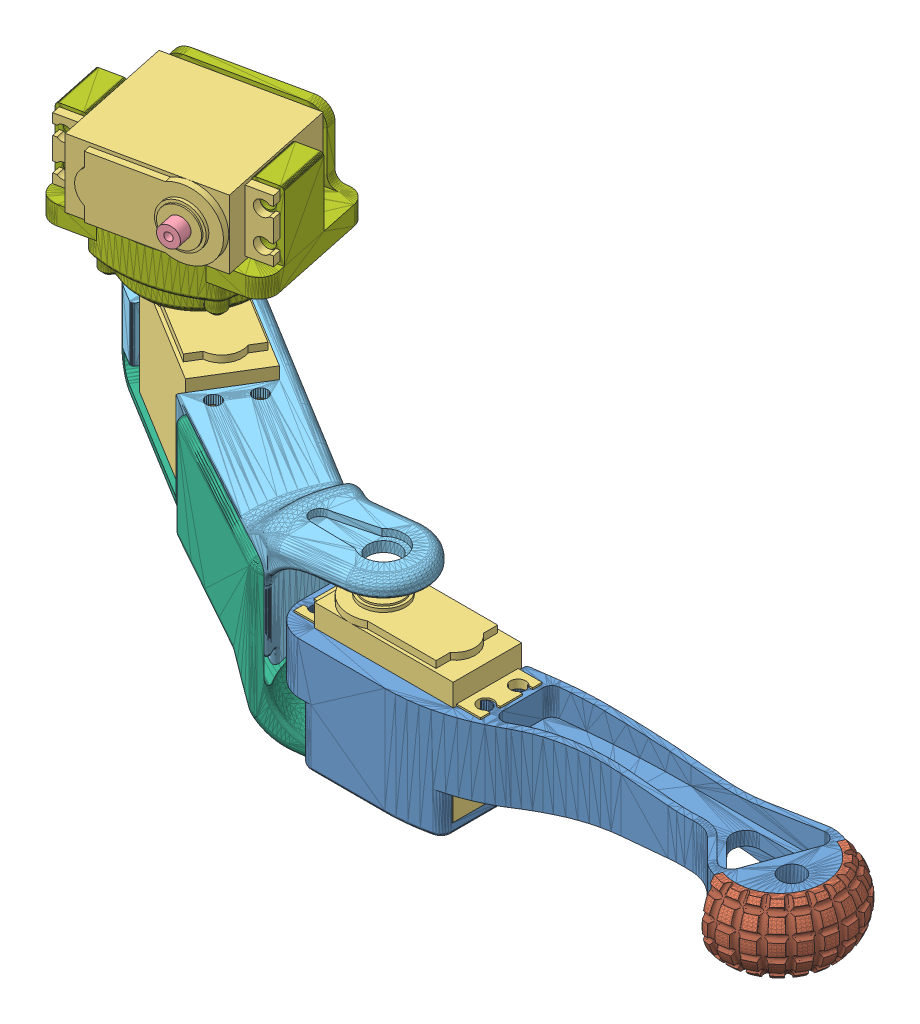
SolidWorks assembly left_foot_front, configuration Default. Lengths in mm.
Overall size (271.86 94.6 110.14).
14 component instances, 7 part files, 22 mates.
Components (placement in the parent):
- L_wrist_mg-1: L_wrist_mg [Default] at (-104.9134 49.2874 139.9903) size (149.99 36.9 30)
- foot-1: foot [Default] at (21.0866 19.2874 149.9903) x (0.342019 0 -0.939693) z (-0.939693 0 -0.342019) size (38.32 20 19.41)
- MG996R-1: MG996R [Default] at (-84.6634 -9.7126 149.9903) size (54.5 43 20)
  - servo-1: servo [Default] at origin size (54.5 39 20)
  - shaft-1: shaft [Default] at (-10.1089 43 0) x (-0.837169 0 -0.546944) z (-0.546944 0 0.837169) size (5.9 19.57 5.9)
- L_arm_mg-1: L_arm_mg [Default] at (-196.4399 30.2874 92.0951) x (-0.522898 0 0.852395) z (0.852395 0 0.522898) size (38.24 39.8 137.4)
- MG996R-2: MG996R [Default] at (-184.4079 -1.7126 111.2077) x (0.852395 0 0.522898) z (-0.522898 0 0.852395) size (54.5 43 20)
  - servo-1: servo [Default] at origin size (54.5 39 20)
  - shaft-1: shaft [Default] at (-10.1089 43 0) x (-0.837169 0 -0.546944) z (-0.546944 0 0.837169) size (5.9 19.57 5.9)
- L_arm_cover-1: L_arm_cover [Default] at (-199.5307 32.5874 83.7466) x (-0.522898 0 0.852395) z (0.852395 0 0.522898) size (41.16 45 143.55)
- MG996R-3: MG996R [Default] at (-196.3785 66.9874 90.0217) x (-0.978469 0 0.206392) z (0 1 0) size (54.5 43 20)
  - servo-1: servo [Default] at origin size (54.5 39 20)
  - shaft-1: shaft [Default] at (-10.1089 43 0) x (-0.837169 0 -0.546944) z (-0.546944 0 0.837169) size (5.9 19.57 5.9)
- R_arm_joint_mg-1: R_arm_joint_mg [Default] at (-214.9542 106.9874 100.0719) x (0 1 0) z (0.978469 0 -0.206392) size (37.5 46 56.5)
Mates (geometry in assembly coordinates):
- Coincident1: coincident anti-aligned: plane of L_wrist_mg-1 through (9.5615 49.2874 181.6556) normal (0.939693 0 0.342019); plane of foot-1 through (21.0866 19.2874 149.9903) normal (-0.939693 0 -0.342019)
- Parallel2: parallel aligned: line of foot-1 through (16.6404 -0.7126 162.2063) axis (0 1 0); line of L_wrist_mg-1 through (16.6404 -0.7126 162.2063) axis (0 1 0)
- Coincident4: coincident: point of foot-1; point of L_wrist_mg-1
- Coincident5: coincident anti-aligned: plane of L_wrist_mg-1 through (-104.9134 49.2874 159.9903) normal (0 0 -1); plane of MG996R-1/servo-1 through (-104.9134 25.7874 159.9903) normal (0 0 1)
- Coincident6: coincident anti-aligned: plane of L_wrist_mg-1 through (-104.9134 -9.7126 139.9903) normal (0 1 0); plane of MG996R-1/servo-1 through (-84.6634 -9.7126 149.9903) normal (0 -1 0)
- Coincident7: coincident anti-aligned: plane of L_wrist_mg-1 through (-64.4134 49.2874 139.9903) normal (-1 0 0); plane of MG996R-1/servo-1 through (-64.4134 25.7874 159.9903) normal (1 0 0)
- Parallel4: parallel aligned: plane of MG996R-1/servo-1 through (-94.7723 27.7874 149.9903) normal (0 1 0); plane of L_arm_mg-1 through (-196.4399 30.2874 92.0951) normal (0 1 0)
- Coincident14: coincident anti-aligned: plane of L_arm_mg-1 through (-196.4399 25.2874 92.0951) normal (0 1 0); plane of MG996R-2/servo-1 through (-202.8078 25.2874 94.3478) normal (0 -1 0)
- Coincident15: coincident anti-aligned: plane of L_arm_mg-1 through (-196.4399 30.2874 92.0951) normal (0.852395 0 0.522898); plane of MG996R-2/servo-1 through (-206.8978 33.7874 109.143) normal (-0.852395 0 -0.522898)
- Coincident16: coincident anti-aligned: plane of L_arm_mg-1 through (-196.4399 30.2874 92.0951) normal (-0.522898 0 0.852395); plane of MG996R-2/servo-1 through (-196.4399 33.7874 92.0951) normal (0.522898 0 -0.852395)
- Coincident18: coincident: line of MG996R-1/shaft-1 through (-94.7723 33.2874 149.9903) axis (0 -1 0)
- Distance1: distance = 2 mm: line of L_arm_mg-1 through (-93.1834 35.2874 154.1881) axis (-0.353984 0 -0.935252)
- Coincident21: coincident anti-aligned: plane of L_arm_cover-1 through (-199.5307 27.7874 83.7466) normal (0 -1 0); plane of MG996R-2/servo-1 through (-202.8078 27.7874 94.3478) normal (0 1 0)
- Parallel5: parallel anti-aligned: plane of MG996R-2/servo-1 through (-206.8978 33.7874 109.143) normal (-0.852395 0 -0.522898); plane of L_arm_cover-1 through (-193.5639 32.5874 87.4069) normal (0.852395 0 0.522898)
- Coincident23: coincident anti-aligned: plane of MG996R-2/servo-1 through (-206.8978 33.7874 109.143) normal (-0.852395 0 -0.522898); plane of L_arm_cover-1 through (-193.5639 32.5874 87.4069) normal (0.852395 0 0.522898)
- Parallel6: parallel aligned: plane of L_arm_mg-1 through (-193.8254 30.2874 87.8331) normal (0.522898 0 -0.852395); plane of L_arm_cover-1 through (-199.5307 32.5874 83.7466) normal (0.522898 0 -0.852395)
- Coincident25: coincident anti-aligned: plane of L_arm_mg-1 through (-196.4399 30.2874 92.0951) normal (-0.522898 0 0.852395); plane of L_arm_cover-1 through (-202.4066 32.5874 88.4348) normal (0.522898 0 -0.852395)
- Coincident26: coincident: line of MG996R-2/shaft-1 through (-193.0246 41.2874 105.9218) axis (0 -1 0)
- Distance2: distance = 1 mm aligned: plane of MG996R-2/shaft-1 through (-193.0246 41.2874 105.9218) normal (0 1 0); plane of R_arm_joint_mg-1 through (-214.9542 42.2874 100.0719) normal (0 1 0)
- Coincident28: coincident anti-aligned: plane of MG996R-3/servo-1 through (-166.8334 62.2374 111.3837) normal (-0.206392 0 -0.978469); plane of R_arm_joint_mg-1 through (-210.6199 106.9874 120.6198) normal (0.206392 0 0.978469)
- Coincident31: coincident anti-aligned: plane of MG996R-3/servo-1 through (-169.2376 56.9874 120.5779) normal (0 -1 0); plane of R_arm_joint_mg-1 through (-214.9542 56.9874 100.0719) normal (0 1 0)
- Coincident32: coincident anti-aligned: plane of MG996R-3/servo-1 through (-169.2376 76.9874 120.5779) normal (0.978469 0 -0.206392); plane of R_arm_joint_mg-1 through (-175.3261 106.9874 91.7131) normal (-0.978469 0 0.206392)
